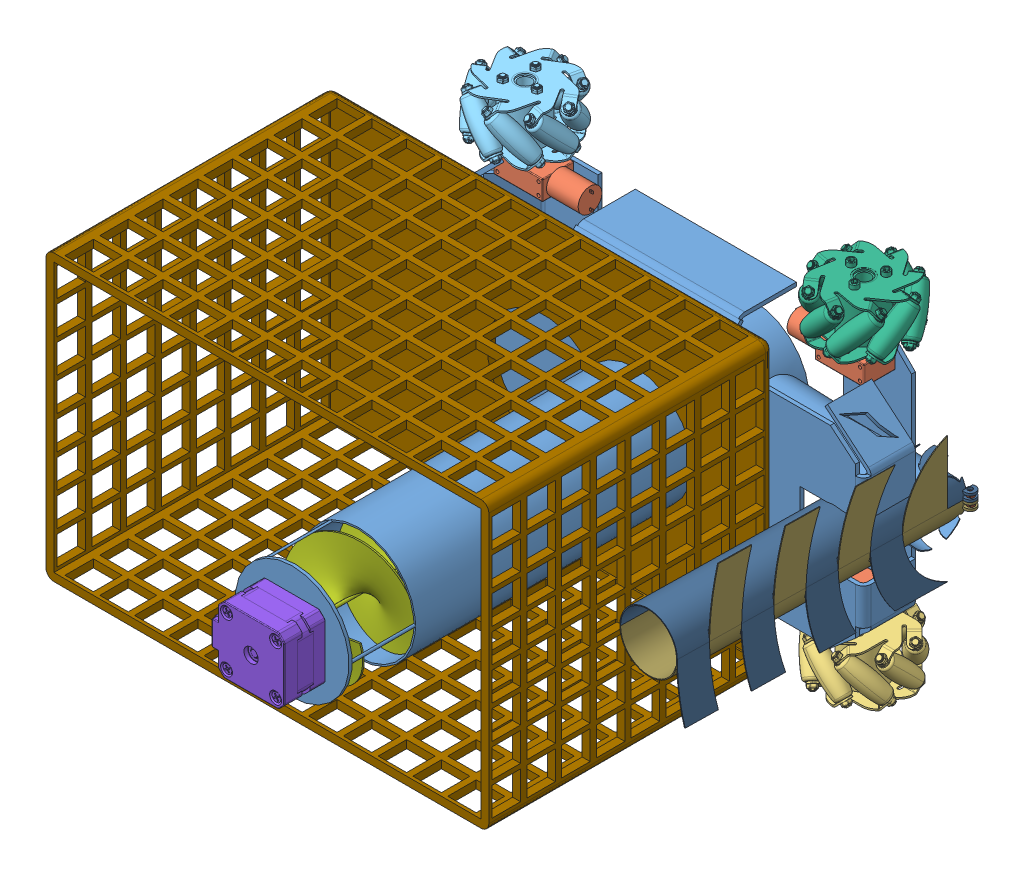
SolidWorks assembly tennis_car3, configuration 默认. Lengths in mm.
Overall size (342.44 226.19 334.2).
20 component instances, 12 part files, 28 mates.
Components (placement in the parent):
- car_main_body-1: car_main_body [默认] at (-145.051 -370.0736 71.4729) x (0 1 0) z (0 0 1) size (155.3 280.48 291.54)
- RF-1: RF [默认] at (73.9859 -396.0617 -100.86) size (72.83 55.75 59.47)
  - DC-1: DC [默认] at (11.5455 -40.5143 8.3808) x (-1 0 0) z (0 -1 0) size (53.09 20 29.75)
  - Mecanum_wheel_RF-1: Mecanum_wheel_RF [默认] at (50.073 -104.5143 -58.7387) x (0 1 0) z (0 0 1) size (37 59.47 59.47)
- RB-1: RB [默认] at (-99.6113 -409.5895 -127.3135) size (85.22 55.84 84.26)
  - DC-1: DC [默认] at (0.8482 -26.9825 34.8343) x (1 0 0) z (0 -1 0) size (53.09 20 29.75)
  - Mecanum_wheel_RB2-1: Mecanum_wheel_RB2 [默认] at (-29.583 -87.0073 9.2199) x (0 -1 0) z (0.536613 0 0.843828) size (37 61.04 61.04)
- LB-1: LB [默认] at (-105.6209 -285.1235 -91.7022) size (78.74 55.75 71.3)
  - DC-1: DC [默认] at (6.8577 -59.4516 -0.777) x (1 0 0) z (0 1 0) size (53.09 20 29.75)
  - Mecanum_wheel_LB2-1: Mecanum_wheel_LB2 [默认] at (-16.0195 4.5484 -71.463) x (0 -1 0) z (-0.224244 0 0.974533) size (37 59.47 59.47)
- LF-1: LF [默认] at (100.0091 -244.6315 -121.7936) size (85.57 55.84 84.97)
  - DC-1: DC [默认] at (-14.4777 -99.9396 29.3144) x (-1 0 0) z (0 1 0) size (53.09 20 29.75)
  - Mecanum_wheel_LF2-1: Mecanum_wheel_LF2 [默认] at (24.6483 -39.9149 11.6464) x (0 1 0) z (-0.82086 0 0.571129) size (37 61.04 61.04)
- spiral_tube-1: spiral_tube [默认] at (4.7184 -390.5736 -116.766) x (0.166187 -0.986094 0) z (0 0 1) size (68 68 282.11)
- Stepper Motor3-1: Stepper Motor3 [默认] at (4.7184 -390.5736 198.234) x (0 1 0) z (-1 0 0) size (42 43 47.1)
- box2-1: box2 [默认] at (-52.9088 -300.5736 41.234) x (1 0 0) z (0 -1 0) size (280 180 180)
- 夹爪-1: 夹爪 [默认] at (126.3983 -390.5736 -113.4559) x (0 1 0) z (-0.017044 0 0.999855) size (58.5 41.56 184.56)
- connection1-1: connection1 [默认] at (140.8179 -393.0736 -113.3823) x (0.999248 0 0.038769) z (0.038769 0 -0.999248) size (9.12 3 4.5)
- connection1-2: connection1 [默认] at (140.8179 -388.0736 -113.3823) x (0.999248 0 0.038769) z (0.038769 0 -0.999248) size (9.12 3 4.5)
- 夹爪2-1: 夹爪2 [默认] at (126.3983 -390.5736 -113.4559) x (0 1 0) z (-0.017044 0 0.999855) size (58.5 41.56 184.56)
Mates (geometry in assembly coordinates):
- 重合1: coincident anti-aligned: plane of RF-1/DC-1 through (110.5314 -436.576 -102.4792) normal (0 0 -1); plane of car_main_body-1 through (100.4806 -390.5736 -102.4792) normal (0 0 1)
- 重合2: coincident aligned: plane of car_main_body-1 through (-145.051 -461.576 71.4729) normal (0 -1 0); plane of RF-1/DC-1 through (85.5314 -461.576 -92.4792) normal (0 -1 0)
- 重合3: coincident: line of car_main_body-1 through (110.5314 -461.576 -104.9792) axis (0 0 1); plane of RF-1/DC-1 through (110.5314 -461.576 -107.4792) normal (1 0 0)
- 重合4: coincident anti-aligned: plane of car_main_body-1 through (-91.0439 -390.5736 -102.4792) normal (0 0 1); plane of RB-1/DC-1 through (-123.7631 -436.5721 -102.4792) normal (0 0 -1)
- 重合5: coincident aligned: plane of car_main_body-1 through (-123.6589 -461.5721 -103.9928) normal (0 -1 0); plane of RB-1/DC-1 through (-98.7631 -461.5721 -92.4792) normal (0 -1 0)
- 重合6: coincident: line of car_main_body-1 through (-123.7631 -445.1021 -102.4792) axis (0 -1 0); plane of RB-1/DC-1 through (-123.7631 -461.5721 -77.4792) normal (-1 0 0)
- 重合7: coincident anti-aligned: plane of car_main_body-1 through (-91.0439 -390.5736 -102.4792) normal (0 0 1); plane of LB-1/DC-1 through (-123.7631 -344.5751 -102.4792) normal (0 0 -1)
- 重合8: coincident aligned: plane of car_main_body-1 through (-125.6782 -319.5751 -101.5862) normal (0 1 0); plane of LB-1/DC-1 through (-98.7631 -319.5751 -92.4792) normal (0 1 0)
- 重合9: coincident: line of car_main_body-1 through (-123.7631 -319.5751 -102.4792) axis (0 -1 0); plane of LB-1/DC-1 through (-123.7631 -319.5751 -107.4792) normal (-1 0 0)
- 重合10: coincident anti-aligned: plane of car_main_body-1 through (100.4806 -390.5736 -102.4792) normal (0 0 1); plane of LF-1/DC-1 through (110.5314 -344.5712 -102.4792) normal (0 0 -1)
- 重合11: coincident aligned: plane of car_main_body-1 through (-145.051 -319.5712 71.4729) normal (0 1 0); plane of LF-1/DC-1 through (85.5314 -319.5712 -92.4792) normal (0 1 0)
- 重合12: coincident: line of car_main_body-1 through (110.5314 -319.5712 -102.4792) axis (0 0 -1); plane of LF-1/DC-1 through (110.5314 -319.5712 -77.4792) normal (1 0 0)
- 同心1: concentric aligned: cylinder of car_main_body-1 through (4.7184 -390.5736 171.234) axis (0 0 -1) radius 36; cylinder of spiral_tube-1 through (4.7184 -390.5736 165.234) axis (0 0 -1) radius 1
- 重合13: coincident anti-aligned: plane of car_main_body-1 through (4.7184 -390.5736 -116.766) normal (0 0 1); plane of spiral_tube-1 through (4.7184 -390.5736 -116.766) normal (0 0 -1)
- 同心2: concentric aligned: cylinder of car_main_body-1 through (4.7184 -390.5736 171.234) axis (0 0 1) radius 11; cylinder of Stepper Motor3-1 through (4.7184 -390.5736 155.234) axis (0 0 1) radius 2.5
- 同心3: concentric aligned: circle of car_main_body-1; cone of Stepper Motor3-1 through (20.2184 -375.0736 173.234) axis (0 0 1)
- 重合16: coincident anti-aligned: plane of car_main_body-1 through (4.7184 -390.5736 173.234) normal (0 0 1); plane of Stepper Motor3-1 through (4.7184 -390.5736 173.234) normal (0 0 -1)
- 重合17: coincident anti-aligned: plane of car_main_body-1 through (4.7184 -390.5736 -48.766) normal (0 0 1); plane of box2-1 through (-192.9088 -480.5736 -48.766) normal (0 0 -1)
- 重合18: coincident aligned: plane of car_main_body-1 through (-145.051 -390.5736 71.4729) normal (0 -1 0); plane of box2-1 through (-52.9088 -390.5736 41.234) normal (0 -1 0)
- 同心4: concentric anti-aligned: cylinder of car_main_body-1 through (129.4557 -393.0736 179.4723) axis (0.038769 0 -0.999248) radius 1; cylinder of connection1-1 through (140.8955 -393.0736 -115.3808) axis (-0.038769 0 0.999248) radius 1
- 重合20: coincident aligned: plane of car_main_body-1 through (140.8955 -393.0736 -115.3808) normal (0.038769 0 -0.999248); plane of connection1-1 through (140.8955 -393.0736 -115.3808) normal (0.038769 0 -0.999248)
- 同心5: concentric anti-aligned: cylinder of car_main_body-1 through (129.4557 -388.0736 179.4723) axis (0.038769 0 -0.999248) radius 1; cylinder of connection1-2 through (140.8955 -388.0736 -115.3808) axis (-0.038769 0 0.999248) radius 1
- 重合22: coincident aligned: plane of car_main_body-1 through (140.8955 -388.0736 -115.3808) normal (0.038769 0 -0.999248); plane of connection1-2 through (140.8955 -388.0736 -115.3808) normal (0.038769 0 -0.999248)
- 重合23: coincident aligned: circle of 夹爪-1; cylinder of connection1-2 through (145.9742 -389.0736 -114.183) axis (0 1 0) radius 1.5
- 重合24: coincident anti-aligned: plane of 夹爪-1 through (145.9742 -389.0736 -114.183) normal (0 1 0); plane of connection1-2 through (145.9742 -389.0736 -114.183) normal (0 -1 0)
- 同心6: concentric aligned: cylinder of 夹爪2-1 through (145.9742 -385.5736 -114.183) axis (0 -1 0) radius 1.5; circle of connection1-1
- 重合26: coincident anti-aligned: plane of connection1-1 through (145.9742 -392.0736 -114.183) normal (0 1 0); plane of 夹爪2-1 through (145.9742 -392.0736 -114.183) normal (0 -1 0)
- 重合27: coincident aligned: plane of 夹爪-1 through (142.1686 -430.5736 46.8362) normal (0.999855 0 0.017044); plane of 夹爪2-1 through (142.5094 -350.5736 26.8391) normal (0.999855 0 0.017044)
